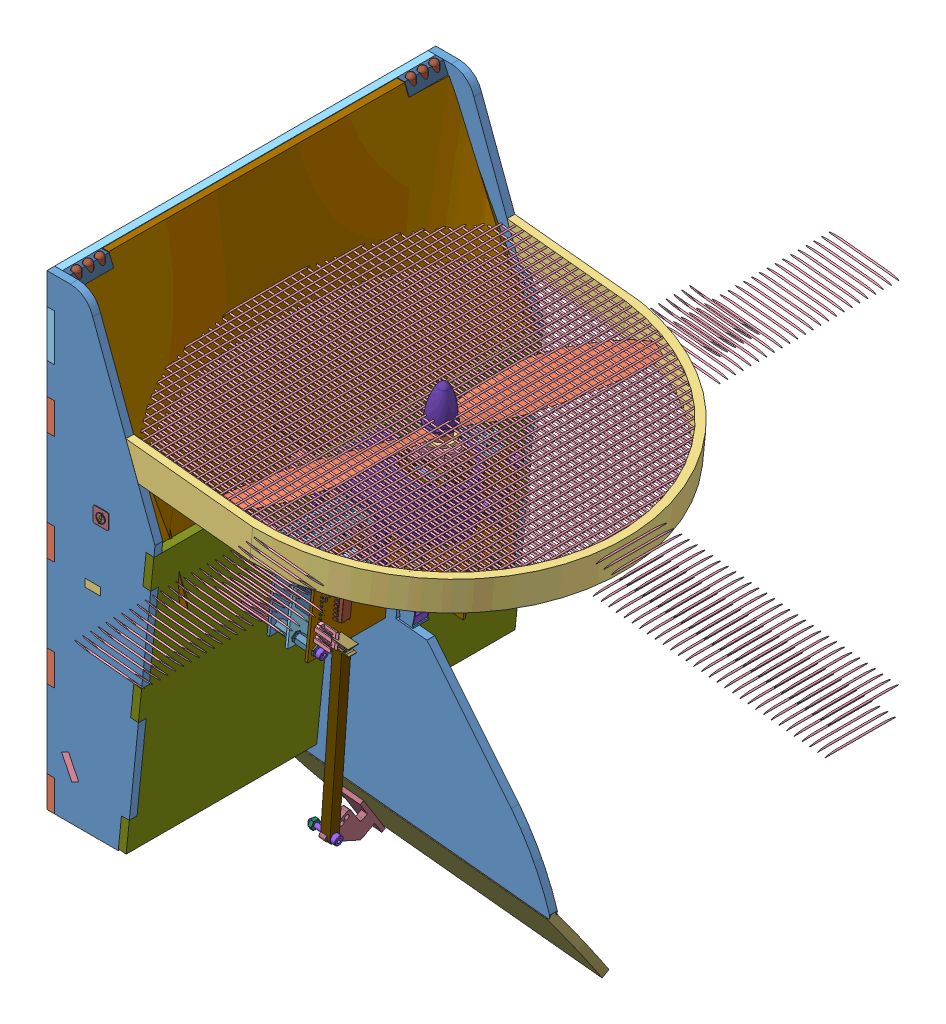
SolidWorks assembly AssTotaleSimu7, configuration Défaut. Lengths in mm. (continued)
Components (placement in the parent): (continued)
- AssStructSimu-1: AssStructSimu [Défaut] at (-125.7658 -1.8483 624.6548) x (1 0 0) z (0 0 -1) size (253.25 324.59 251.6) (continued)
  - AssCarte-1: AssCarte [Défaut] at (38.0121 147.1029 290.772) x (-0.101852 0.9948 0) z (0.9948 0.101852 0) size (66.52 130.57 98.72) (continued)
    - AssEntretoise-3: AssEntretoise [Défaut] at (-106.8199 -51.2976 37.1344) x (0 0 -1) z (1 0 0) size (58.24 7.29 7.81)
      - socket head cap screw 4762_din-1: socket head cap screw 4762_din [EN ISO 4762 M3 x 5 - 5N] at (-2.4967 0.5867 0) size (8 5.5 5.5)
      - hexagonal_spacer_MF_M3_H20_HEX5.5_FTD6_MTL6-1: hexagonal_spacer_MF_M3_H20_HEX5.5_FTD6_MTL6 [Défaut] at (48.3433 0.5867 0) x (0 0 1) z (-1 0 0) size (6.36 5.51 26)
      - hex nut style 1 gradeab_din-1: hex nut style 1 gradeab_din [Hexagon Nut ISO 4032 - M3 - W - N] at (53.3433 0.5867 0) x (0 0.943962 0.330053) z (-1 0 0) size (5.5 6.35 2.4)
      - hexagonal_spacer_MF_M3_H12_HEX5.5_FTD6_MTL6-2: hexagonal_spacer_MF_M3_H12_HEX5.5_FTD6_MTL6 [Défaut] at (27.0633 0.5867 0) x (0 0.248308 0.968681) z (-1 0 0) size (6.36 5.51 18)
      - hexagonal_spacer_MF_M3_H12_HEX5.5_FTD6_MTL6-3: hexagonal_spacer_MF_M3_H12_HEX5.5_FTD6_MTL6 [Défaut] at (13.7833 0.5867 0) x (0 0 1) z (-1 0 0) size (6.36 5.51 18)
    - AssEntretoise-4: AssEntretoise [Défaut] at (-106.8199 68.7024 37.1344) x (0 0 -1) z (1 0 0) size (58.24 7.29 7.81)
      - socket head cap screw 4762_din-1: socket head cap screw 4762_din [EN ISO 4762 M3 x 5 - 5N] at (-2.4967 0.5867 0) size (8 5.5 5.5)
      - hexagonal_spacer_MF_M3_H20_HEX5.5_FTD6_MTL6-1: hexagonal_spacer_MF_M3_H20_HEX5.5_FTD6_MTL6 [Défaut] at (48.3433 0.5867 0) x (0 0 1) z (-1 0 0) size (6.36 5.51 26)
      - hex nut style 1 gradeab_din-1: hex nut style 1 gradeab_din [Hexagon Nut ISO 4032 - M3 - W - N] at (53.3433 0.5867 0) x (0 0.943962 0.330053) z (-1 0 0) size (5.5 6.35 2.4)
      - hexagonal_spacer_MF_M3_H12_HEX5.5_FTD6_MTL6-2: hexagonal_spacer_MF_M3_H12_HEX5.5_FTD6_MTL6 [Défaut] at (27.0633 0.5867 0) x (0 0.248308 0.968681) z (-1 0 0) size (6.36 5.51 18)
      - hexagonal_spacer_MF_M3_H12_HEX5.5_FTD6_MTL6-3: hexagonal_spacer_MF_M3_H12_HEX5.5_FTD6_MTL6 [Défaut] at (13.7833 0.5867 0) x (0 0 1) z (-1 0 0) size (6.36 5.51 18)
    - AssMpu-1: AssMpu [Défaut] at (-150.6881 40.5798 29.6372) x (0.908747 0.417347 0) z (0 0 1) size (8 8 22.28)
      - hex nut style 1 gradeab_din-1: hex nut style 1 gradeab_din [Hexagon Nut ISO 4032 - M3 - W - N] at (0.2783 0.3227 1.2) size (5.5 6.35 2.4)
      - plain washer 6903 type ab_din-1: plain washer 6903 type ab_din [DIN 6903-A3] at (0.2783 0.3227 1.2) x (0 0 1) z (-1 0 0) size (1 8 8)
      - socket head cap screw 4762_din-1: socket head cap screw 4762_din [EN ISO 4762 M3 x 5 - 5N] at (0.2783 0.3227 19.76) x (0 0 -1) z (-0.852155 0.523289 0) size (8 5.5 5.5)
      - hexagonal_spacer_MF_M3_H12_HEX5.5_FTD6_MTL6-1: hexagonal_spacer_MF_M3_H12_HEX5.5_FTD6_MTL6 [Défaut] at (0.2783 0.3227 3.48) size (6.36 5.51 18)
    - AssMpu-2: AssMpu [Défaut] at (-130.3481 40.6665 29.6372) size (8 8 22.28)
      - hex nut style 1 gradeab_din-1: hex nut style 1 gradeab_din [Hexagon Nut ISO 4032 - M3 - W - N] at (0.2783 0.3227 1.2) size (5.5 6.35 2.4)
      - plain washer 6903 type ab_din-1: plain washer 6903 type ab_din [DIN 6903-A3] at (0.2783 0.3227 1.2) x (0 0 1) z (-1 0 0) size (1 8 8)
      - socket head cap screw 4762_din-1: socket head cap screw 4762_din [EN ISO 4762 M3 x 5 - 5N] at (0.2783 0.3227 19.76) x (0 0 -1) z (-0.852155 0.523289 0) size (8 5.5 5.5)
      - hexagonal_spacer_MF_M3_H12_HEX5.5_FTD6_MTL6-1: hexagonal_spacer_MF_M3_H12_HEX5.5_FTD6_MTL6 [Défaut] at (0.2783 0.3227 3.48) size (6.36 5.51 18)
    - AssCosse-1: AssCosse [Défaut] at (-142.6764 26.8797 71.168) x (0 -1 0) z (-0.344896 0 -0.938641) size (9.83 18.66 11.64)
      - socket head cap screw 4762_din-1: socket head cap screw 4762_din [EN ISO 4762 M3 x 6 - 6N] at (-5.1064 0.3659 0) size (9 5.5 5.5)
      - plain washer 6903 type ab_din-1: plain washer 6903 type ab_din [DIN 6903-A3] at (-2.1064 0.3659 0) size (1 8 8)
      - hex nut style 1 gradeab_din-2: hex nut style 1 gradeab_din [Hexagon Nut ISO 4032 - M3 - W - N] at (1.281 0.3659 0) x (0 0.924225 0.381849) z (-1 0 0) size (5.5 6.35 2.4)
      - 31880-1: 31880 [Default] at (0.4936 0.3659 0) x (0 0.344896 -0.938641) z (0 -0.938641 -0.344896) size (5.54 5 17.37)
    - AssCosse-2: AssCosse [Défaut] at (-142.6764 -2.9203 71.168) x (0 -1 0) z (-0.344896 0 -0.938641) size (9.83 18.66 11.64)
      - socket head cap screw 4762_din-1: socket head cap screw 4762_din [EN ISO 4762 M3 x 6 - 6N] at (-5.1064 0.3659 0) size (9 5.5 5.5)
      - plain washer 6903 type ab_din-1: plain washer 6903 type ab_din [DIN 6903-A3] at (-2.1064 0.3659 0) size (1 8 8)
      - hex nut style 1 gradeab_din-2: hex nut style 1 gradeab_din [Hexagon Nut ISO 4032 - M3 - W - N] at (1.281 0.3659 0) x (0 0.924225 0.381849) z (-1 0 0) size (5.5 6.35 2.4)
      - 31880-1: 31880 [Default] at (0.4936 0.3659 0) x (0 0.344896 -0.938641) z (0 -0.938641 -0.344896) size (5.54 5 17.37)
    - AssCosse-3: AssCosse [Défaut] at (-142.6764 12.0797 71.168) x (0 -1 0) z (-0.344896 0 -0.938641) size (9.83 18.66 11.64)
      - socket head cap screw 4762_din-1: socket head cap screw 4762_din [EN ISO 4762 M3 x 6 - 6N] at (-5.1064 0.3659 0) size (9 5.5 5.5)
      - plain washer 6903 type ab_din-1: plain washer 6903 type ab_din [DIN 6903-A3] at (-2.1064 0.3659 0) size (1 8 8)
      - hex nut style 1 gradeab_din-2: hex nut style 1 gradeab_din [Hexagon Nut ISO 4032 - M3 - W - N] at (1.281 0.3659 0) x (0 0.924225 0.381849) z (-1 0 0) size (5.5 6.35 2.4)
      - 31880-1: 31880 [Default] at (0.4936 0.3659 0) x (0 0.344896 -0.938641) z (0 -0.938641 -0.344896) size (5.54 5 17.37)
    - Terminal_QD_Female-1: Terminal_QD_Female [Default] at (-137.2199 31.5422 53.3942) x (0 1 0) z (-1 0 0) size (9.4 5.5 22.35)
    - Terminal_QD_Female-2: Terminal_QD_Female [Default] at (-137.3199 31.5422 36.2942) x (0 -1 0) z (-1 0 0) size (9.4 5.5 22.35)
    - Terminal_QD_Female-3: Terminal_QD_Female [Default] at (-137.2199 1.7422 53.3942) x (0 1 0) z (-1 0 0) size (9.4 5.5 22.35)
    - Terminal_QD_Female-4: Terminal_QD_Female [Default] at (-137.3199 1.7422 35.9942) x (0 1 0) z (-1 0 0) size (9.4 5.5 22.35)
    - Terminal_QD_Female-5: Terminal_QD_Female [Default] at (-137.3199 16.7422 35.9942) x (0 1 0) z (-1 0 0) size (9.4 5.5 22.35)
    - Terminal_QD_Female-6: Terminal_QD_Female [Default] at (-137.2199 16.7422 53.3942) x (0 1 0) z (-1 0 0) size (9.4 5.5 22.35)
- AssTige-1: AssTige [Défaut] at (-241.576 -121.7726 340.4233) x (-0.101791 -0.994204 -0.034587) z (0.9948 -0.101852 0) size (166.39 7.19 19)
  - tige_servo-1: tige_servo [Défaut] at (-106.2712 0.2685 162) size (165 6 6)
  - socket head cap screw 4762_din-2: socket head cap screw 4762_din [EN ISO 4762 M2 x 10 - 10N] at (-104.2712 3.2685 170) x (0 0 -1) z (0.923728 0.383049 0) size (12 3.8 3.8)
  - hex nut style 1 gradeab_din-1: hex nut style 1 gradeab_din [Hexagon Nut ISO 4032 - M3 - W - N] at (55.7288 3.2685 156) size (5.5 6.35 2.4)
  - hex nut style 1 gradeab_din-2: hex nut style 1 gradeab_din [Hexagon Nut ISO 4032 - M2 - W - N] at (-104.2712 3.2685 160) x (0.904801 0.425836 0) z (0 0 1) size (4 4.62 1.6)
  - socket head cap screw 4762_din-3: socket head cap screw 4762_din [EN ISO 4762 M3 x 16 - 16N] at (55.7288 3.2685 171) x (0 0 -1) z (0.923728 0.383049 0) size (19 5.5 5.5)
- AssGoPro-1: AssGoPro [Défaut] at (-119.9926 15.1708 318.2917) x (0 0 -1) z (-0.119031 -0.99289 0) size (64.3 52.3 34.42)
  - GoPRo Frame for LCD Screen-1: GoPRo Frame for LCD Screen [Défaut] at (-2.6935 10.9558 5.5635) size (64.3 47.42 34.42)
    - GoProFrame MJM-1: GoProFrame MJM [Défaut] at (-3.6084 -1.6692 52.45) size (64.3 59.3 23.5)
    - GoPro Hero 3 Front Panel-1: GoPro Hero 3 Front Panel [Défaut] at (-3.6084 -1.6692 55.7) x (-1 0 0) z (0 0 -1) size (59.25 41.2 1.9)
    - GoPro Hero 3 Screen-1: GoPro Hero 3 Screen [Défaut] at (12.7166 3.9308 54.9) size (15 18 1)
    - GoPro Hero 3 Mode Button-1: GoPro Hero 3 Mode Button [Défaut] at (13.4166 -12.4692 54.95) x (-1 0 0) z (0 0 -1) size (11.97 12.11 3.03)
    - GoPro Hero 3 LED Cover-1: GoPro Hero 3 LED Cover [Défaut] at (3.1166 -9.3192 54.85) x (-0.999988 0.004848 0) z (0 0 -1) size (5 5 1.4)
    - GoPro Hero 3 LED Cover-2: GoPro Hero 3 LED Cover [Défaut] at (3.1166 -16.0692 54.85) x (-0.999988 0.004848 0) z (0 0 -1) size (5 5 1.4)
    - GoPro Hero 3 Housing-1: GoPro Hero 3 Housing [Défaut] at (-3.6084 -1.6692 55.7) size (59.37 41.3 29.84)
    - GoPro Hero 3 Lens-1: GoPro Hero 3 Lens [Défaut] at (-18.9334 5.6308 47.35) x (-0.380542 -0.924764 0) z (0 0 -1) size (13.71 15.7 7.94)
    - GoPro Hero 3 Indicator Cover-1: GoPro Hero 3 Indicator Cover [Défaut] at (-25.5834 -22.2692 69.9) x (-0.997412 0 -0.0719) z (0 1 0) size (3 3 2)
    - GoPro Hero 3 Indicator Cover-2: GoPro Hero 3 Indicator Cover [Défaut] at (-28.8834 12.2308 73) x (-0.999992 0.004018 0) z (0 0 1) size (3 3 2)
    - GoPro Hero 3 Indicator Cover-3: GoPro Hero 3 Indicator Cover [Défaut] at (20.6666 16.9308 58.4) x (-0.997739 0 -0.067212) z (0 1 0) size (3 3 2)
    - slot-1: slot [Défaut] at (-24.7434 -9.7363 65.05) x (0 1 0) z (0 0 -1) size (16 15.02 2.44)
    - GoPro Hero 3 HDMI pin-1: GoPro Hero 3 HDMI pin [Défaut] at (-26.982 2.9815 24.7172) x (0.105491 0.98175 -0.158237) z (-0.992872 0.095109 -0.071829) size (3.29 0.86 3.28)
  - support1-2: support1 [Défaut] at (-1.3019 -18.8633 67.0135) x (0 0 1) z (-1 0 0) size (5 5 10)
- AssGouv-1: AssGouv [Défaut] at (-43.2668 -298.2106 479.8345) x (0.9948 -0.101852 0) z (0.055947 0.546439 -0.835628) size (200.18 52.5 43.47)
  - P10_1-1: P10_1 [Défaut] at (-108.1667 -19.4144 197.6829) size (200.18 50.13 5)
  - attache_pale-1: attache_pale [Défaut] at (-49.1667 8.0856 190.1829) x (0 0 -1) z (-1 0 0) size (43.47 35 14)
- Parallax-Servo-Horn-1: Parallax-Servo-Horn [Défaut] at (-69.3162 -29.8353 324.5606) x (0.09792 0.956393 0.27518) z (0.9948 -0.101852 0) size (38.81 38.81 6.17)
- NTM_35-36_engine_assembly-1: NTM_35-36_engine_assembly [Défaut] at (-24.3523 26.8781 325.7101) x (0.9948 -0.101852 0) z (0 0 1) size (60.56 77.2 246.41)
  - engine_base-1: engine_base [Défaut] at (-1.8719 -19.5526 -1.1165) x (0 1 0) z (0 0 1) size (6.8 35 35)
  - engine_bearing-1: engine_bearing [Défaut] at origin size (10 4 10)
  - Propeller_cone-1: Propeller_cone [Défaut] at (-1.8719 33.6474 -4.1165) x (1 0 0) z (0 1 0) size (17.6 17.6 24)
  - engine_bearing-2: engine_bearing [Défaut] at (0 22.8 0) size (10 4 10)
  - NTM_35-36_enginebody-1: NTM_35-36_enginebody [Défaut] at (-1.8719 -12.7526 -1.1165) size (35 31.7 35)
  - Stator-1: Stator [Défaut] at origin size (27.75 22.36 27.94)
  - propellers_10x4-1: propellers_10x4 [Défaut] at (-6.8719 27.4474 -4.9165) size (60.56 10.53 246.41)
  - propeller_washer-1: propeller_washer [Défaut] at (-1.8719 24.4474 -1.1165) x (0 1 0) z (0 0 1) size (2.5 18 18)
  - Propeller_adaptor-1: Propeller_adaptor [Défaut] at (2.1948 17.1101 -3.713) size (23.46 32.5 25)
Mates (geometry in assembly coordinates):
- Coaxiale1: concentric aligned: cylinder of AssStructSimu-1/AssToitMot-1/AssToit-1/P12-1 through (-27.6967 12.5918 324.5936) axis (-0.101852 -0.9948 0) radius 17.5; cylinder of NTM_35-36_engine_assembly-1/NTM_35-36_enginebody-1 through (-25.2217 36.7654 324.5936) axis (-0.101852 -0.9948 0) radius 17.5
- Coïncidente1: coincident anti-aligned: plane of AssStructSimu-1/AssToitMot-1/AssToit-1/P12-1 through (-28.206 7.6178 324.5936) normal (0.101852 0.9948 0); plane of NTM_35-36_engine_assembly-1/engine_bearing-1 through (-28.206 7.6178 324.5936) normal (-0.101852 -0.9948 0)
- Coaxiale2: concentric aligned: cylinder of AssStructSimu-1/AssToitMot-1/AssToit-1/P10_2-1 through (49.7135 -178.7878 324.5936) axis (-0.9948 0.101852 0) radius 2.5; cylinder of AssGouv-1/P10_1-1 through (-94.0351 -164.0702 324.5936) axis (-0.9948 0.101852 0) radius 2.5
- Coïncidente2: coincident aligned: plane of AssStructSimu-1/AssToitMot-1/AssToit-1/P10_2-1 through (-137.5516 -157.1017 322.0936) normal (-0.9948 0.101852 0); plane of AssGouv-1/P10_1-1 through (-137.8791 -160.3008 321.1312) normal (-0.9948 0.101852 0)
- Coaxiale3: concentric aligned: cylinder of AssTige-1/socket head cap screw 4762_din-3 through (-45.5416 -197.7164 335.2292) axis (0.9948 -0.101852 0) radius 1.5; cylinder of AssGouv-1/attache_pale-1 through (-85.9983 -193.5742 335.2292) axis (0.9948 -0.101852 0) radius 1.5
- Coaxiale4: concentric aligned: cylinder of AssStructSimu-1/AssToitMot-1/Parallax-Servo_DUMMY-1 through (-70.6554 -29.6982 324.5606) axis (-0.9948 0.101852 0) radius 2.9845; cylinder of Parallax-Servo-Horn-1 through (-70.6554 -29.6982 324.5606) axis (-0.9948 0.101852 0) radius 2.9845
- Coïncidente3: coincident anti-aligned: plane of AssStructSimu-1/AssToitMot-1/Parallax-Servo_DUMMY-1 through (-74.8246 -29.2713 324.5606) normal (0.9948 -0.101852 0); plane of Parallax-Servo-Horn-1 through (-74.8246 -29.2713 324.5606) normal (-0.9948 0.101852 0)
- Coaxiale5: concentric anti-aligned: cylinder of AssTige-1/socket head cap screw 4762_din-2 through (-30.2498 -38.5418 340.7631) axis (0.9948 -0.101852 0) radius 1; cylinder of Parallax-Servo-Horn-1 through (-69.7931 -34.4932 340.7631) axis (-0.9948 0.101852 0) radius 0.635
- Coïncidente4: coincident anti-aligned: plane of AssTige-1/tige_servo-1 through (-69.6001 -32.608 343.8305) normal (-0.9948 0.101852 0); plane of Parallax-Servo-Horn-1 through (-68.8748 -25.5237 332.3708) normal (0.9948 -0.101852 0)
- Coaxiale6: concentric aligned: cylinder of AssStructSimu-1/AssBase-1/socket head cap screw 4762_din-7 through (-144.5139 -51.9008 369.3436) axis (0 0 1) radius 1.5; cylinder of AssGoPro-1/support1-2 through (-144.5139 -51.9008 319.5936) axis (0 0 1) radius 1.5
- Coïncidente5: coincident anti-aligned: plane of AssStructSimu-1/AssBase-1/support2-1 through (-141.9706 -54.3568 329.5936) normal (0 0 -1); plane of AssGoPro-1/support1-2 through (-146.6985 -49.121 329.5936) normal (0 0 1)
